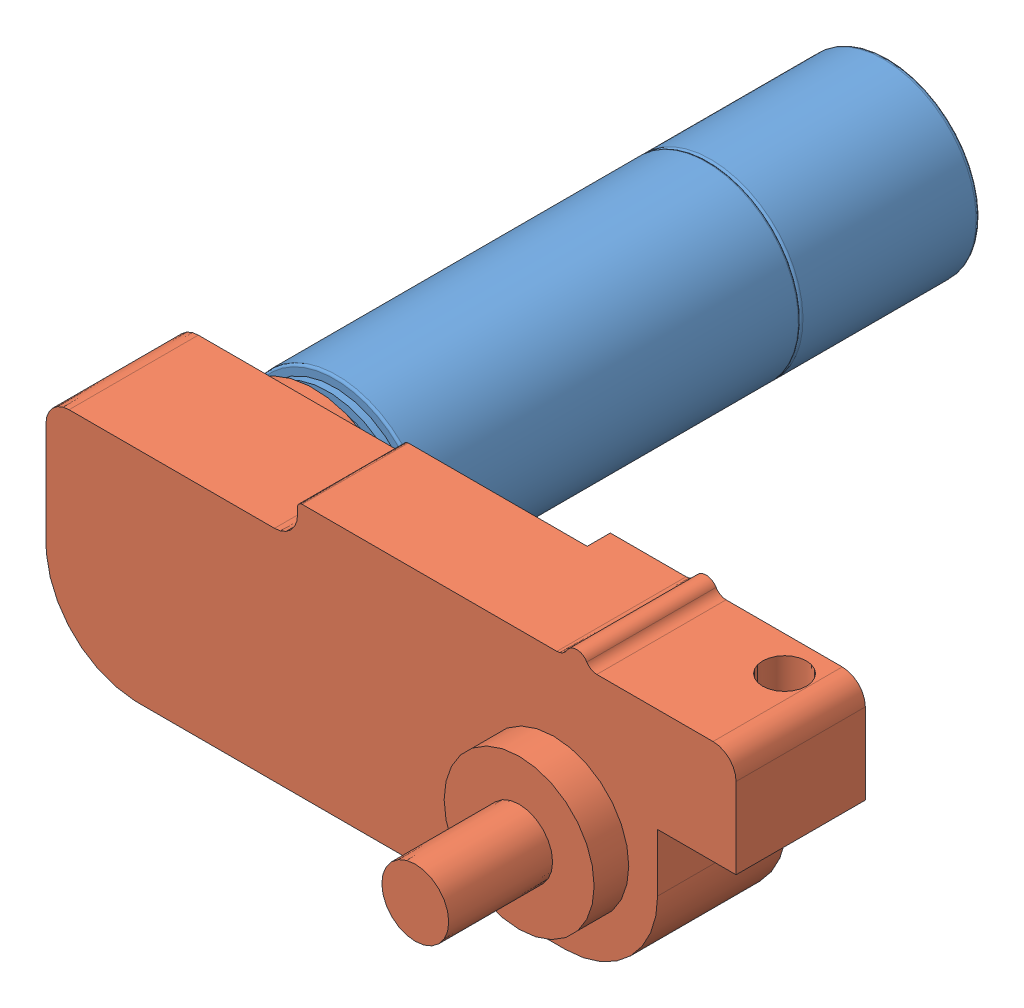
SolidWorks assembly PA2-50_with_gearbox, configuration Default. Lengths in mm.
Overall size (30.92 12.52 38.5).
2 component instances, 2 part files, 2 mates.
Components (placement in the parent):
- PA2-50-1: PA2-50 [Default] at (26.117 -19.7771 -19.1) x (0 0 1) z (0.954024 0.299729 0) size (29.1 8 8)
- gearbox-1: gearbox [Default] at origin size (29.9 11.5 13.6)
Mates (geometry in assembly coordinates):
- Concentric1: concentric anti-aligned: cylinder of PA2-50-1 through (33.0734 -1.5025 -2.9) axis (0 0 -1) radius 4; cylinder of gearbox-1 through (33.0734 -1.5025 -2) axis (0 0 1) radius 4
- Distance1: distance = 0.9 mm anti-aligned: plane of PA2-50-1 through (33.0734 -1.5025 -2.9) normal (0 0 1); plane of gearbox-1 through (33.0734 -1.5025 -2) normal (0 0 -1)
